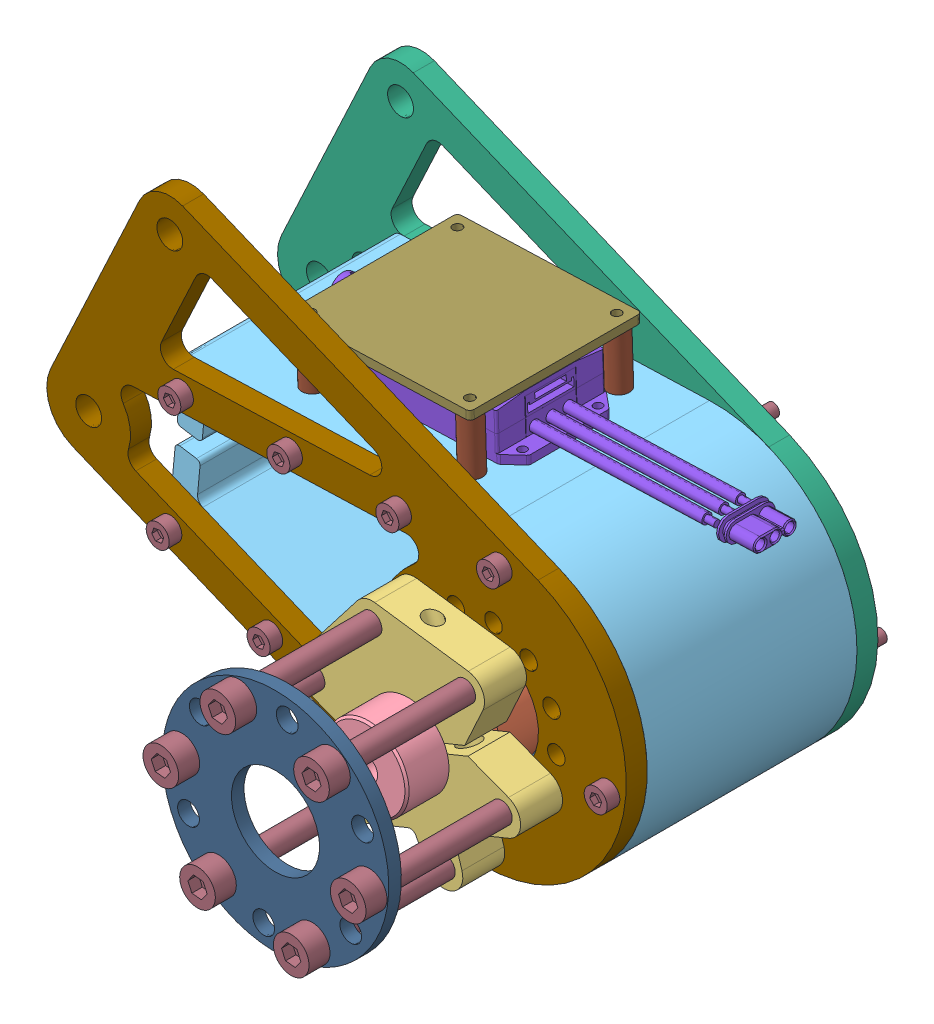
SolidWorks assembly DP_左旋轮组_1, configuration 默认. Lengths in mm.
Overall size (149.92 108.23 130.7).
38 component instances, 14 part files, 81 mates.
Components (placement in the parent):
- DP_RoboMaster GM3508无刷减速电机-1: DP_RoboMaster GM3508无刷减速电机 [默认] at origin size (42 44.98 98.4)
- DP_左旋_mecanum_wheel-1: DP_左旋_mecanum_wheel [默认] at (53.5328 61.8586 -71.6518) x (0.97528 -0.220971 0) z (0 0 1) size (152.18 152.18 48.1) (hidden)
- DP_10x24x9_推力球轴承-1: DP_10x24x9_推力球轴承 [默认] at (34.8209 73.9788 29.9) size (24 24 10)
- DP_夹紧联轴器2-1: DP_夹紧联轴器2 [默认] at (34.8209 73.9788 34.9) x (-0.925598 -0.378508 0) z (0 0 1) size (47.97 54.2 10)
- DP_轮组端盖_1-1: DP_轮组端盖_1 [默认] at (34.8209 73.9788 44.9) size (19.5 19.5 10)
- DP_轮组打印件垫块_1-1: DP_轮组打印件垫块_1 [默认] at (-59.3094 86.804 21.9) x (-0.990845 0.135002 0) z (0 0 -1) size (114.05 68 50)
- DP_轮组电机保护板_1-1: DP_轮组电机保护板_1 [默认] at (-59.3094 86.804 -28.1) x (-0.990845 0.135002 0) z (0 0 -1) size (139 90.3 5)
- DP_滚花铜螺母M2x5-1: DP_滚花铜螺母M2x5 [默认] at (23.1661 107.604 -12.1) x (0.865887 0.029289 0.499381) z (0.033806 -0.999428 0) size (3 3 5)
- DP_滚花铜螺母M2x5-2: DP_滚花铜螺母M2x5 [默认] at (23.1661 107.604 5.9) x (0.956367 0.032349 0.290373) z (0.033806 -0.999428 0) size (3 3 5)
- DP_滚花铜螺母M2x5-3: DP_滚花铜螺母M2x5 [默认] at (-22.0081 106.076 -12.1) x (0.998099 0.033761 0.051554) z (0.033806 -0.999428 0) size (3 3 5)
- DP_滚花铜螺母M2x5-4: DP_滚花铜螺母M2x5 [默认] at (-22.0081 106.076 5.9) x (0.980312 0.033159 -0.194652) z (0.033806 -0.999428 0) size (3 3 5)
- DP_C620无刷电机调速器-1: DP_C620无刷电机调速器 [默认] at (2.0954 112.2944 -3.1) x (0.999428 0.033806 0) z (0 0 -1) size (103.05 11.5 26.13)
- DP_轮组电机安装板_1-2: DP_轮组电机安装板_1 [默认] at (-59.3094 86.804 26.9) x (-0.990845 0.135002 0) z (0 0 -1) size (139 90.3 5)
- DP_轮毂挡板_1-1: DP_轮毂挡板_1 [默认] at (34.8209 73.9788 73.5004) x (0.921464 0.388463 0) z (0 0 1) size (54 54 3)
- DP_滚花铜螺母M2x5-5: DP_滚花铜螺母M2x5 [默认] at (19.5681 107.4823 14.4) x (0.956367 0.032349 0.290373) z (0.033806 -0.999428 0) size (3 3 5)
- DP_滚花铜螺母M2x5-6: DP_滚花铜螺母M2x5 [默认] at (-18.2411 101.2005 14.4) x (0.960301 0.032482 0.277069) z (-0.033806 0.999428 0) size (3 3 5)
- DP_滚花铜螺母M2x5-7: DP_滚花铜螺母M2x5 [默认] at (-18.4102 106.1977 -20.6) x (-0.956367 -0.032349 -0.290373) z (0.033806 -0.999428 0) size (3 3 5)
- DP_滚花铜螺母M2x5-8: DP_滚花铜螺母M2x5 [默认] at (19.5681 107.4823 -20.6) x (-0.956367 -0.032349 -0.290373) z (0.033806 -0.999428 0) size (3 3 5)
- DP_垫高柱-1: DP_垫高柱 [默认] at (19.3484 113.9786 -20.6) x (0.919005 0.031085 -0.393019) z (0.033806 -0.999428 0) size (5 5 13)
- DP_垫高柱-2: DP_垫高柱 [默认] at (19.3484 113.9786 14.4) x (0.919005 0.031085 -0.393019) z (0.033806 -0.999428 0) size (5 5 13)
- DP_垫高柱-3: DP_垫高柱 [默认] at (-18.6299 112.694 14.4) x (0.919005 0.031085 -0.393019) z (0.033806 -0.999428 0) size (5 5 13)
- DP_垫高柱-4: DP_垫高柱 [默认] at (-18.6299 112.694 -20.6) x (0.919005 0.031085 -0.393019) z (0.033806 -0.999428 0) size (5 5 13)
- DP_亚克力保护-1: DP_亚克力保护 [默认] at (0.1395 119.8326 -3.1) x (0.999428 0.033806 0) z (-0.033806 0.999428 0) size (44 41 2)
- DP_圆柱头螺栓-1: DP_圆柱头螺栓 [M5*40] at (43.5613 53.2458 76.5004) x (0.409196 -0.912446 0) z (-0.912446 -0.409196 0) size (8.5 45 8.5)
- DP_圆柱头螺栓-2: DP_圆柱头螺栓 [M5*40] at (21.2358 56.0429 76.5004) x (0.409196 -0.912446 0) z (-0.912446 -0.409196 0) size (8.5 45 8.5)
- DP_圆柱头螺栓-3: DP_圆柱头螺栓 [M5*40] at (12.4954 76.7758 76.5004) x (0.409196 -0.912446 0) z (-0.912446 -0.409196 0) size (8.5 45 8.5)
- DP_圆柱头螺栓-4: DP_圆柱头螺栓 [M5*40] at (26.0804 94.7117 76.5004) x (0.409196 -0.912446 0) z (-0.912446 -0.409196 0) size (8.5 45 8.5)
- DP_圆柱头螺栓-5: DP_圆柱头螺栓 [M5*40] at (48.4059 91.9147 76.5004) x (0.409196 -0.912446 0) z (-0.912446 -0.409196 0) size (8.5 45 8.5)
- DP_圆柱头螺栓-6: DP_圆柱头螺栓 [M5*40] at (57.1463 71.1817 76.5004) x (0.409196 -0.912446 0) z (-0.912446 -0.409196 0) size (8.5 45 8.5)
- DP_圆柱头螺栓-7: DP_圆柱头螺栓 [M3*65] at (30.7708 44.2534 26.9) x (0.983587 0.180432 0) z (0.180432 -0.983587 0) size (5.5 68 5.5)
- DP_圆柱头螺栓-8: DP_圆柱头螺栓 [M3*65] at (8.228 52.4888 26.9) x (0.983587 0.180432 0) z (0.180432 -0.983587 0) size (5.5 68 5.5)
- DP_圆柱头螺栓-9: DP_圆柱头螺栓 [M3*65] at (-15.8116 62.3932 26.9) x (0.983587 0.180432 0) z (0.180432 -0.983587 0) size (5.5 68 5.5)
- DP_圆柱头螺栓-10: DP_圆柱头螺栓 [M3*65] at (-39.8512 72.2977 26.9) x (0.983587 0.180432 0) z (0.180432 -0.983587 0) size (5.5 68 5.5)
- DP_圆柱头螺栓-11: DP_圆柱头螺栓 [M3*65] at (-37.0963 101.5633 26.9) x (0.983587 0.180432 0) z (0.180432 -0.983587 0) size (5.5 68 5.5)
- DP_圆柱头螺栓-12: DP_圆柱头螺栓 [M3*65] at (-11.1112 102.4423 26.9) x (0.983587 0.180432 0) z (0.180432 -0.983587 0) size (5.5 68 5.5)
- DP_圆柱头螺栓-13: DP_圆柱头螺栓 [M3*65] at (14.874 103.3212 26.9) x (0.983587 0.180432 0) z (0.180432 -0.983587 0) size (5.5 68 5.5)
- DP_圆柱头螺栓-14: DP_圆柱头螺栓 [M3*65] at (38.8709 103.7041 26.9) x (0.983587 0.180432 0) z (0.180432 -0.983587 0) size (5.5 68 5.5)
- DP_圆柱头螺栓-15: DP_圆柱头螺栓 [M3*65] at (64.5462 69.9287 26.9) x (0.983587 0.180432 0) z (0.180432 -0.983587 0) size (5.5 68 5.5)
Mates (geometry in assembly coordinates):
- 同心1: concentric anti-aligned: cylinder of RoboMaster GM3508无刷减速电机-1 through (34.8209 73.9788 49.2) axis (0 0 1) radius 5; cylinder of 10x24x9_推力球轴承-1 through (34.8209 73.9788 34.9) axis (0 0 -1) radius 5
- 重合1: coincident anti-aligned: plane of RoboMaster GM3508无刷减速电机-1 through (34.8209 73.9788 24.9) normal (0 0 1); plane of 10x24x9_推力球轴承-1 through (34.8209 73.9788 24.9) normal (0 0 -1)
- 同心2: concentric anti-aligned: cylinder of RoboMaster GM3508无刷减速电机-1 through (34.8209 73.9788 49.2) axis (0 0 1) radius 5; cylinder of 夹紧联轴器2-1 through (34.8209 73.9788 44.9) axis (0 0 -1) radius 5
- 重合2: coincident anti-aligned: plane of 10x24x9_推力球轴承-1 through (34.8209 73.9788 34.9) normal (0 0 1); plane of 夹紧联轴器2-1 through (34.8209 73.9788 34.9) normal (0 0 -1)
- 重合3: coincident anti-aligned: plane of 夹紧联轴器2-1 through (34.8209 73.9788 44.9) normal (0 0 1); plane of DP_轮组端盖_1-1 through (34.8209 73.9788 44.9) normal (0 0 -1)
- 同心3: concentric anti-aligned: cylinder of RoboMaster GM3508无刷减速电机-1 through (34.8209 73.9788 49.2) axis (0 0 1) radius 5; cylinder of DP_轮组端盖_1-1 through (34.8209 73.9788 54.9) axis (0 0 -1) radius 9.75
- 重合4: coincident anti-aligned: plane of RoboMaster GM3508无刷减速电机-1 through (36.0836 78.8167 29.2) normal (-0.378508 0.925598 0); plane of 夹紧联轴器2-1 through (36.0836 78.8167 44.9) normal (0.378508 -0.925598 0)
- 重合5: coincident anti-aligned: plane of 左旋_mecanum_wheel-1 through (34.8209 73.9788 44.9) normal (0 0 -1); plane of 夹紧联轴器2-1 through (57.1527 70.8487 44.9) normal (0 0 1)
- 同心4: concentric anti-aligned: cylinder of 左旋_mecanum_wheel-1 through (34.8209 73.9788 33.8264) axis (0 0 1) radius 10; cylinder of 10x24x9_推力球轴承-1 through (34.8209 73.9788 34.9) axis (0 0 -1) radius 12
- 同心11: concentric aligned: cylinder of DP_轮组打印件垫块_1-1 through (23.9774 83.6177 -12.1) axis (-0.033806 0.999428 0) radius 1.6; cylinder of 滚花铜螺母M2x5-1 through (23.3351 102.6069 -12.1) axis (-0.033806 0.999428 0) radius 1.5
- 重合9: coincident aligned: plane of DP_轮组打印件垫块_1-1 through (33.6715 107.9594 117.2572) normal (-0.033806 0.999428 0); plane of 滚花铜螺母M2x5-1 through (23.1661 107.604 -12.1) normal (-0.033806 0.999428 0)
- 重合10: coincident aligned: plane of DP_轮组打印件垫块_1-1 through (33.6715 107.9594 117.2572) normal (-0.033806 0.999428 0); plane of 滚花铜螺母M2x5-2 through (23.1661 107.604 5.9) normal (-0.033806 0.999428 0)
- 同心12: concentric aligned: cylinder of DP_轮组打印件垫块_1-1 through (23.9774 83.6177 5.9) axis (-0.033806 0.999428 0) radius 1.6; cylinder of 滚花铜螺母M2x5-2 through (23.3351 102.6069 5.9) axis (-0.033806 0.999428 0) radius 1.5
- 重合11: coincident aligned: plane of DP_轮组打印件垫块_1-1 through (33.6715 107.9594 117.2572) normal (-0.033806 0.999428 0); plane of 滚花铜螺母M2x5-3 through (-22.0081 106.076 -12.1) normal (-0.033806 0.999428 0)
- 同心13: concentric aligned: cylinder of DP_轮组打印件垫块_1-1 through (-21.1968 82.0897 -12.1) axis (-0.033806 0.999428 0) radius 1.6; cylinder of 滚花铜螺母M2x5-3 through (-21.8391 101.0788 -12.1) axis (-0.033806 0.999428 0) radius 1.5
- 重合12: coincident aligned: plane of DP_轮组打印件垫块_1-1 through (33.6715 107.9594 117.2572) normal (-0.033806 0.999428 0); plane of 滚花铜螺母M2x5-4 through (-22.0081 106.076 5.9) normal (-0.033806 0.999428 0)
- 同心14: concentric aligned: cylinder of DP_轮组打印件垫块_1-1 through (-21.1968 82.0897 5.9) axis (-0.033806 0.999428 0) radius 1.6; cylinder of 滚花铜螺母M2x5-4 through (-21.8391 101.0788 5.9) axis (-0.033806 0.999428 0) radius 1.5
- 重合13: coincident anti-aligned: plane of DP_轮组打印件垫块_1-1 through (33.6715 107.9594 117.2572) normal (-0.033806 0.999428 0); plane of DP_C620无刷电机调速器-1 through (0.579 106.84 -3.1) normal (0.033806 -0.999428 0)
- 同心15: concentric aligned: cylinder of 滚花铜螺母M2x5-4 through (-22.0081 106.076 5.9) axis (-0.033806 0.999428 0) radius 0.8; cylinder of DP_C620无刷电机调速器-1 through (-21.687 96.5814 5.9) axis (-0.033806 0.999428 0) radius 1
- 同心16: concentric aligned: cylinder of 滚花铜螺母M2x5-3 through (-22.0081 106.076 -12.1) axis (-0.033806 0.999428 0) radius 0.8; cylinder of DP_C620无刷电机调速器-1 through (-21.687 96.5814 -12.1) axis (-0.033806 0.999428 0) radius 1
- 同心17: concentric anti-aligned: cylinder of 10x24x9_推力球轴承-1 through (34.8209 73.9788 34.9) axis (0 0 -1) radius 12; cylinder of DP_轮组电机安装板_1-2 through (34.8209 73.9788 21.9) axis (0 0 1) radius 34
- 同心18: concentric aligned: cylinder of DP_轮组电机保护板_1-1 through (34.8209 73.9788 -33.1) axis (0 0 1) radius 34; cylinder of DP_轮组电机安装板_1-2 through (34.8209 73.9788 21.9) axis (0 0 1) radius 34
- 同心19: concentric anti-aligned: cylinder of RoboMaster GM3508无刷减速电机-1 through (34.8209 73.9788 -14.1) axis (0 0 -1) radius 21; cylinder of DP_轮组打印件垫块_1-1 through (34.8209 73.9788 -28.1) axis (0 0 1) radius 34
- 重合15: coincident anti-aligned: plane of RoboMaster GM3508无刷减速电机-1 through (29.7918 61.9909 21.9) normal (0 0 1); plane of DP_轮组电机安装板_1-2 through (-59.3094 86.804 21.9) normal (0 0 -1)
- 重合16: coincident anti-aligned: plane of DP_轮组打印件垫块_1-1 through (34.8209 73.9788 21.9) normal (0 0 1); plane of DP_轮组电机安装板_1-2 through (-59.3094 86.804 21.9) normal (0 0 -1)
- 重合17: coincident anti-aligned: plane of DP_轮组打印件垫块_1-1 through (34.8209 73.9788 -28.1) normal (0 0 -1); plane of DP_轮组电机保护板_1-1 through (34.8209 73.9788 -28.1) normal (0 0 1)
- 同心20: concentric anti-aligned: cylinder of RoboMaster GM3508无刷减速电机-1 through (18.6229 67.3549 21.9) axis (0 0 1) radius 1.65; cylinder of DP_轮组电机安装板_1-2 through (18.6229 67.3549 55.9) axis (0 0 -1) radius 2.1
- 平行1: parallel aligned: plane of DP_轮组电机保护板_1-1 through (47.7725 105.4153 -33.1) normal (0.380931 0.924603 0); plane of DP_轮组电机安装板_1-2 through (-37.2158 140.43 21.9) normal (0.380931 0.924603 0)
- 同心21: concentric aligned: cylinder of DP_轮组打印件垫块_1-1 through (-37.0963 101.5633 39.9) axis (0 0 -1) radius 1.6; cylinder of DP_轮组电机安装板_1-2 through (-37.0963 101.5633 45.9) axis (0 0 -1) radius 1.6
- 重合18: coincident anti-aligned: plane of 左旋_mecanum_wheel-1 through (34.8209 73.9788 73.5004) normal (0 0 1); plane of 轮毂挡板_1-1 through (34.8209 73.9788 73.5004) normal (0 0 -1)
- 同心22: concentric anti-aligned: cylinder of 左旋_mecanum_wheel-1 through (43.5613 53.2458 73.5004) axis (0 0 1) radius 2.6; cylinder of 轮毂挡板_1-1 through (43.5613 53.2458 76.5004) axis (0 0 -1) radius 2.6
- 同心23: concentric aligned: cylinder of 左旋_mecanum_wheel-1 through (34.8209 73.9788 84.574) axis (0 0 -1) radius 10; cylinder of 轮毂挡板_1-1 through (34.8209 73.9788 76.5004) axis (0 0 -1) radius 10.5
- 同心24: concentric aligned: cylinder of DP_轮组打印件垫块_1-1 through (19.9062 97.488 14.4) axis (-0.033806 0.999428 0) radius 1.6; cylinder of 滚花铜螺母M2x5-5 through (19.5681 107.4823 14.4) axis (-0.033806 0.999428 0) radius 0.8
- 重合19: coincident aligned: plane of DP_轮组打印件垫块_1-1 through (33.6715 107.9594 117.2572) normal (-0.033806 0.999428 0); plane of 滚花铜螺母M2x5-5 through (19.5681 107.4823 14.4) normal (-0.033806 0.999428 0)
- 同心251: concentric anti-aligned: cylinder of DP_轮组打印件垫块_1-1 through (-18.0721 96.2034 14.4) axis (-0.033806 0.999428 0) radius 1.6; cylinder of 滚花铜螺母M2x5-6 through (-18.4102 106.1977 14.4) axis (0.033806 -0.999428 0) radius 1.5
- 重合21: coincident aligned: plane of DP_轮组打印件垫块_1-1 through (33.6715 107.9594 117.2572) normal (-0.033806 0.999428 0); plane of 滚花铜螺母M2x5-6 through (-18.4102 106.1977 14.4) normal (-0.033806 0.999428 0)
- 同心261: concentric aligned: cylinder of DP_轮组打印件垫块_1-1 through (-18.0721 96.2034 -20.6) axis (-0.033806 0.999428 0) radius 1.6; cylinder of 滚花铜螺母M2x5-7 through (-18.4102 106.1977 -20.6) axis (-0.033806 0.999428 0) radius 0.8
- 重合22: coincident aligned: plane of DP_轮组打印件垫块_1-1 through (33.6715 107.9594 117.2572) normal (-0.033806 0.999428 0); plane of 滚花铜螺母M2x5-7 through (-18.4102 106.1977 -20.6) normal (-0.033806 0.999428 0)
- 同心271: concentric aligned: cylinder of DP_轮组打印件垫块_1-1 through (19.9062 97.488 -20.6) axis (-0.033806 0.999428 0) radius 1.6; cylinder of 滚花铜螺母M2x5-8 through (19.5681 107.4823 -20.6) axis (-0.033806 0.999428 0) radius 0.8
- 重合23: coincident aligned: plane of DP_轮组打印件垫块_1-1 through (33.6715 107.9594 117.2572) normal (-0.033806 0.999428 0); plane of 滚花铜螺母M2x5-8 through (19.5681 107.4823 -20.6) normal (-0.033806 0.999428 0)
- 重合24: coincident anti-aligned: plane of DP_轮组打印件垫块_1-1 through (33.6715 107.9594 117.2572) normal (-0.033806 0.999428 0); plane of DP_垫高柱-1 through (19.5681 107.4823 -20.6) normal (0.033806 -0.999428 0)
- 同心28: concentric aligned: cylinder of 滚花铜螺母M2x5-8 through (19.5681 107.4823 -20.6) axis (-0.033806 0.999428 0) radius 0.8; cylinder of DP_垫高柱-1 through (19.5681 107.4823 -20.6) axis (-0.033806 0.999428 0) radius 2.5
- 同心291: concentric aligned: cylinder of DP_轮组打印件垫块_1-1 through (19.9062 97.488 14.4) axis (-0.033806 0.999428 0) radius 1.6; cylinder of DP_垫高柱-2 through (19.5681 107.4823 14.4) axis (-0.033806 0.999428 0) radius 2.5
- 重合251: coincident anti-aligned: plane of DP_轮组打印件垫块_1-1 through (33.6715 107.9594 117.2572) normal (-0.033806 0.999428 0); plane of DP_垫高柱-2 through (19.5681 107.4823 14.4) normal (0.033806 -0.999428 0)
- 同心301: concentric aligned: cylinder of DP_轮组打印件垫块_1-1 through (-18.0721 96.2034 14.4) axis (-0.033806 0.999428 0) radius 1.6; cylinder of DP_垫高柱-3 through (-18.4102 106.1977 14.4) axis (-0.033806 0.999428 0) radius 2.5
- 重合261: coincident anti-aligned: plane of DP_轮组打印件垫块_1-1 through (33.6715 107.9594 117.2572) normal (-0.033806 0.999428 0); plane of DP_垫高柱-3 through (-18.4102 106.1977 14.4) normal (0.033806 -0.999428 0)
- 同心311: concentric aligned: cylinder of 滚花铜螺母M2x5-7 through (-18.4102 106.1977 -20.6) axis (-0.033806 0.999428 0) radius 0.8; cylinder of DP_垫高柱-4 through (-18.4102 106.1977 -20.6) axis (-0.033806 0.999428 0) radius 2.5
- 重合271: coincident anti-aligned: plane of 滚花铜螺母M2x5-7 through (-18.4102 106.1977 -20.6) normal (-0.033806 0.999428 0); plane of DP_垫高柱-4 through (-18.4102 106.1977 -20.6) normal (0.033806 -0.999428 0)
- 重合28: coincident anti-aligned: plane of DP_垫高柱-1 through (19.1286 120.4749 -20.6) normal (-0.033806 0.999428 0); plane of DP_亚克力保护-1 through (0.1395 119.8326 -3.1) normal (0.033806 -0.999428 0)
- 同心32: concentric aligned: cylinder of DP_垫高柱-1 through (19.5681 107.4823 -20.6) axis (-0.033806 0.999428 0) radius 1.5; cylinder of DP_亚克力保护-1 through (19.1286 120.4749 -20.6) axis (-0.033806 0.999428 0) radius 1.1
- 同心33: concentric aligned: cylinder of DP_垫高柱-4 through (-18.4102 106.1977 -20.6) axis (-0.033806 0.999428 0) radius 1.5; cylinder of DP_亚克力保护-1 through (-18.8496 119.1903 -20.6) axis (-0.033806 0.999428 0) radius 1.1
- 同心312: concentric anti-aligned: cylinder of DP_轮毂挡板_1-1 through (43.5613 53.2458 76.5004) axis (0 0 -1) radius 2.6; cylinder of DP_圆柱头螺栓-1 through (43.5613 53.2458 36.5004) axis (0 0 1) radius 2.5
- 重合272: coincident anti-aligned: plane of DP_轮毂挡板_1-1 through (34.8209 73.9788 76.5004) normal (0 0 1); plane of DP_圆柱头螺栓-1 through (43.5613 53.2458 76.5004) normal (0 0 -1)
- 同心3131: concentric aligned: cylinder of DP_轮毂挡板_1-1 through (21.2358 56.0429 76.5004) axis (0 0 -1) radius 2.6; cylinder of DP_圆柱头螺栓-2 through (21.2358 56.0429 81.5004) axis (0 0 -1) radius 4.25
- 重合2731: coincident anti-aligned: plane of DP_轮毂挡板_1-1 through (34.8209 73.9788 76.5004) normal (0 0 1); plane of DP_圆柱头螺栓-2 through (21.2358 56.0429 76.5004) normal (0 0 -1)
- 同心3141: concentric aligned: cylinder of DP_轮毂挡板_1-1 through (12.4954 76.7758 76.5004) axis (0 0 -1) radius 2.6; cylinder of DP_圆柱头螺栓-3 through (12.4954 76.7758 81.5004) axis (0 0 -1) radius 4.25
- 重合2741: coincident anti-aligned: plane of DP_轮毂挡板_1-1 through (34.8209 73.9788 76.5004) normal (0 0 1); plane of DP_圆柱头螺栓-3 through (12.4954 76.7758 76.5004) normal (0 0 -1)
- 同心3151: concentric aligned: cylinder of DP_轮毂挡板_1-1 through (26.0804 94.7117 76.5004) axis (0 0 -1) radius 2.6; cylinder of DP_圆柱头螺栓-4 through (26.0804 94.7117 81.5004) axis (0 0 -1) radius 4.25
- 重合2751: coincident anti-aligned: plane of DP_轮毂挡板_1-1 through (34.8209 73.9788 76.5004) normal (0 0 1); plane of DP_圆柱头螺栓-4 through (26.0804 94.7117 76.5004) normal (0 0 -1)
- 同心3161: concentric aligned: cylinder of DP_轮毂挡板_1-1 through (48.4059 91.9147 76.5004) axis (0 0 -1) radius 2.6; cylinder of DP_圆柱头螺栓-5 through (48.4059 91.9147 81.5004) axis (0 0 -1) radius 4.25
- 重合2761: coincident anti-aligned: plane of DP_轮毂挡板_1-1 through (34.8209 73.9788 76.5004) normal (0 0 1); plane of DP_圆柱头螺栓-5 through (48.4059 91.9147 76.5004) normal (0 0 -1)
- 同心3171: concentric aligned: cylinder of DP_轮毂挡板_1-1 through (57.1463 71.1817 76.5004) axis (0 0 -1) radius 2.6; cylinder of DP_圆柱头螺栓-6 through (57.1463 71.1817 81.5004) axis (0 0 -1) radius 4.25
- 重合2771: coincident anti-aligned: plane of DP_轮毂挡板_1-1 through (34.8209 73.9788 76.5004) normal (0 0 1); plane of DP_圆柱头螺栓-6 through (57.1463 71.1817 76.5004) normal (0 0 -1)
- 同心318: concentric anti-aligned: circle of DP_轮组电机安装板_1-2; cylinder of DP_圆柱头螺栓-7 through (30.7708 44.2534 -38.1) axis (0 0 1) radius 1.5
- 重合278: coincident anti-aligned: plane of DP_轮组电机安装板_1-2 through (-59.3094 86.804 26.9) normal (0 0 1); plane of DP_圆柱头螺栓-7 through (30.7708 44.2534 26.9) normal (0 0 -1)
- 同心3191: concentric aligned: cylinder of DP_轮组电机安装板_1-2 through (8.228 52.4888 45.9) axis (0 0 -1) radius 1.6; cylinder of DP_圆柱头螺栓-8 through (8.228 52.4888 29.9) axis (0 0 -1) radius 2.75
- 重合2791: coincident anti-aligned: plane of DP_轮组电机安装板_1-2 through (-59.3094 86.804 26.9) normal (0 0 1); plane of DP_圆柱头螺栓-8 through (8.228 52.4888 26.9) normal (0 0 -1)
- 同心3201: concentric aligned: cylinder of DP_轮组电机安装板_1-2 through (-15.8116 62.3932 45.9) axis (0 0 -1) radius 1.6; cylinder of DP_圆柱头螺栓-9 through (-15.8116 62.3932 29.9) axis (0 0 -1) radius 2.75
- 重合2801: coincident anti-aligned: plane of DP_轮组电机安装板_1-2 through (-59.3094 86.804 26.9) normal (0 0 1); plane of DP_圆柱头螺栓-9 through (-15.8116 62.3932 26.9) normal (0 0 -1)
- 同心3211: concentric aligned: cylinder of DP_轮组电机安装板_1-2 through (-39.8512 72.2977 45.9) axis (0 0 -1) radius 1.6; cylinder of DP_圆柱头螺栓-10 through (-39.8512 72.2977 29.9) axis (0 0 -1) radius 2.75
- 重合2811: coincident anti-aligned: plane of DP_轮组电机安装板_1-2 through (-59.3094 86.804 26.9) normal (0 0 1); plane of DP_圆柱头螺栓-10 through (-39.8512 72.2977 26.9) normal (0 0 -1)
- 同心3221: concentric aligned: cylinder of DP_轮组电机安装板_1-2 through (-37.0963 101.5633 45.9) axis (0 0 -1) radius 1.6; cylinder of DP_圆柱头螺栓-11 through (-37.0963 101.5633 29.9) axis (0 0 -1) radius 2.75
- 重合2821: coincident anti-aligned: plane of DP_轮组电机安装板_1-2 through (-59.3094 86.804 26.9) normal (0 0 1); plane of DP_圆柱头螺栓-11 through (-37.0963 101.5633 26.9) normal (0 0 -1)
- 同心3231: concentric aligned: cylinder of DP_轮组电机安装板_1-2 through (-11.1112 102.4423 45.9) axis (0 0 -1) radius 1.6; cylinder of DP_圆柱头螺栓-12 through (-11.1112 102.4423 29.9) axis (0 0 -1) radius 2.75
- 重合2831: coincident anti-aligned: plane of DP_轮组电机安装板_1-2 through (-59.3094 86.804 26.9) normal (0 0 1); plane of DP_圆柱头螺栓-12 through (-11.1112 102.4423 26.9) normal (0 0 -1)
- 同心3241: concentric aligned: cylinder of DP_轮组电机安装板_1-2 through (14.874 103.3212 45.9) axis (0 0 -1) radius 1.6; cylinder of DP_圆柱头螺栓-13 through (14.874 103.3212 29.9) axis (0 0 -1) radius 2.75
- 重合2841: coincident anti-aligned: plane of DP_轮组电机安装板_1-2 through (-59.3094 86.804 26.9) normal (0 0 1); plane of DP_圆柱头螺栓-13 through (14.874 103.3212 26.9) normal (0 0 -1)
- 同心3251: concentric anti-aligned: cylinder of DP_轮组电机安装板_1-2 through (38.8709 103.7041 21.9) axis (0 0 1) radius 1.6; cylinder of DP_圆柱头螺栓-14 through (38.8709 103.7041 29.9) axis (0 0 -1) radius 2.75
- 重合2851: coincident anti-aligned: plane of DP_轮组电机安装板_1-2 through (-59.3094 86.804 26.9) normal (0 0 1); plane of DP_圆柱头螺栓-14 through (38.8709 103.7041 26.9) normal (0 0 -1)
- 同心3261: concentric anti-aligned: cylinder of DP_轮组电机安装板_1-2 through (64.5462 69.9287 21.9) axis (0 0 1) radius 1.6; cylinder of DP_圆柱头螺栓-15 through (64.5462 69.9287 29.9) axis (0 0 -1) radius 2.75
- 重合2861: coincident anti-aligned: plane of DP_轮组电机安装板_1-2 through (-59.3094 86.804 26.9) normal (0 0 1); plane of DP_圆柱头螺栓-15 through (64.5462 69.9287 26.9) normal (0 0 -1)
